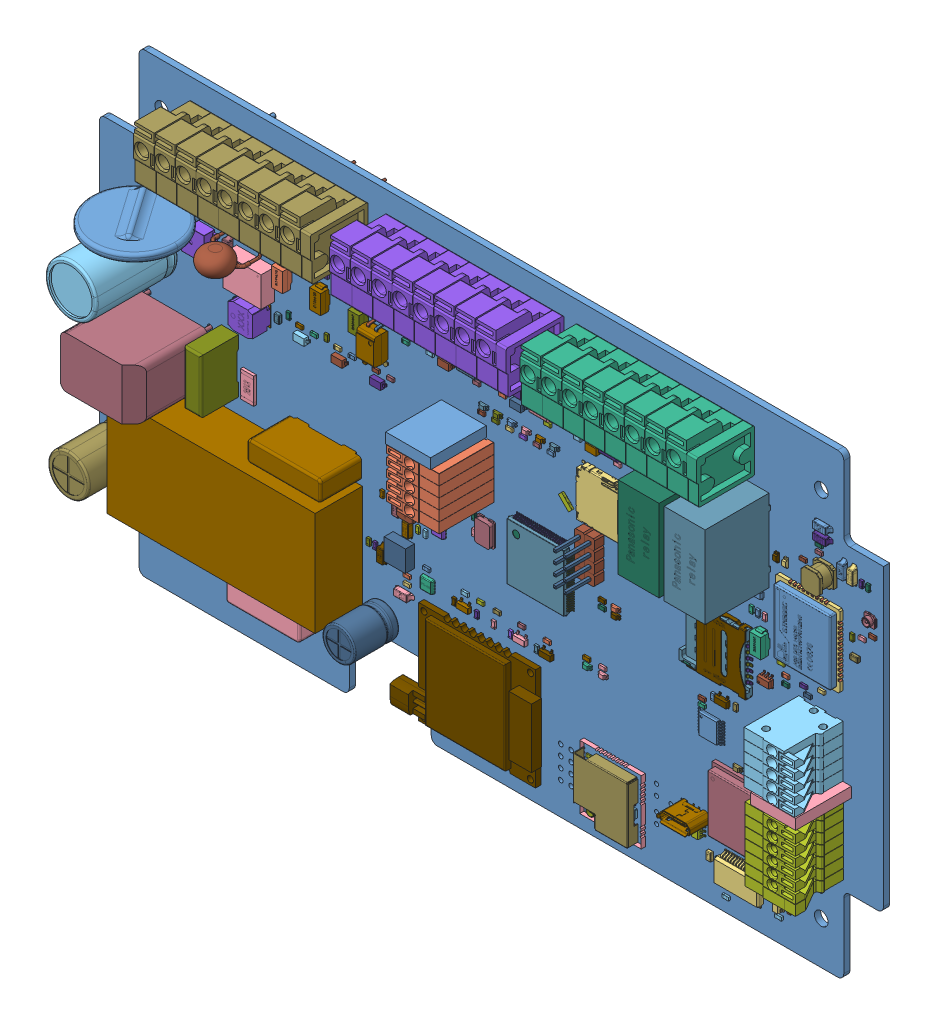
SolidWorks assembly Velvet_Controller_V1.2_2023, configuration Default. Lengths in mm. (continued)
Components (placement in the parent): (continued)
- Velvet_Controller_V1.2_2023(2)^Velvet_Controller_V1.2_2023-1: Velvet_Controller_V1.2_2023(2)^Velvet_Controller_V1.2_2023 [Default] at origin size (191.4 111.4 51.25) (virtual) (continued)
  - C4lr^Velvet_Controller_V1.2_2023(2)_Velvet_Controller_V1.2_2023-1: C4lr^Velvet_Controller_V1.2_2023(2)_Velvet_Controller_V1.2_2023 [Default] at origin size (1.6 0.8 0.5) (virtual)
    - CAP 0603 (1608)^C4lr_Velvet_Controller_V1.2_2023(2)_Velvet_Controller_V1.2_2023-1: CAP 0603 (1608)^C4lr_Velvet_Controller_V1.2_2023(2)_Velvet_Controller_V1.2_2023 [Default] at (130.48 19.301 -1.5) x (-1 0 0) z (0 -1 0) size (1.6 0.5 0.8) (virtual)
  - C4gs^Velvet_Controller_V1.2_2023(2)_Velvet_Controller_V1.2_2023-1: C4gs^Velvet_Controller_V1.2_2023(2)_Velvet_Controller_V1.2_2023 [Default] at origin size (0.8 1.6 0.5) (virtual)
    - CAP 0603 (1608)^C4gs_Velvet_Controller_V1.2_2023(2)_Velvet_Controller_V1.2_2023-1: CAP 0603 (1608)^C4gs_Velvet_Controller_V1.2_2023(2)_Velvet_Controller_V1.2_2023 [Default] at (176.025 78.275 -1.5) x (0 -1 0) z (1 0 0) size (1.6 0.5 0.8) (virtual)
  - C3wf^Velvet_Controller_V1.2_2023(2)_Velvet_Controller_V1.2_2023-1: C3wf^Velvet_Controller_V1.2_2023(2)_Velvet_Controller_V1.2_2023 [Default] at origin size (1.62 4.56 1.51) (virtual)
    - CAP 1206^C3wf_Velvet_Controller_V1.2_2023(2)_Velvet_Controller_V1.2_2023-1: CAP 1206^C3wf_Velvet_Controller_V1.2_2023(2)_Velvet_Controller_V1.2_2023 [Default] at (162.3 28.55 -1.5) x (0 1 0) z (0 0 -1) size (4.56 1.62 1.51) (virtual)
  - C3p^Velvet_Controller_V1.2_2023(2)_Velvet_Controller_V1.2_2023-1: C3p^Velvet_Controller_V1.2_2023(2)_Velvet_Controller_V1.2_2023 [Default] at origin size (8 8 28.5) (virtual)
    - ECA-1HM101B^C3p_Velvet_Controller_V1.2_2023(2)_Velvet_Controller_V1.2_2023-1: ECA-1HM101B^C3p_Velvet_Controller_V1.2_2023(2)_Velvet_Controller_V1.2_2023 [Default] at (69.9 20.9 0) x (0 -1 0) z (-1 0 0) size (8 28.5 8) (virtual)
  - C3mc^Velvet_Controller_V1.2_2023(2)_Velvet_Controller_V1.2_2023-1: C3mc^Velvet_Controller_V1.2_2023(2)_Velvet_Controller_V1.2_2023 [Default] at origin size (1.6 0.8 0.5) (virtual)
    - CAP 0603 (1608)^C3mc_Velvet_Controller_V1.2_2023(2)_Velvet_Controller_V1.2_2023-1: CAP 0603 (1608)^C3mc_Velvet_Controller_V1.2_2023(2)_Velvet_Controller_V1.2_2023 [Default] at (146.575 42.225 0) x (1 0 0) z (0 -1 0) size (1.6 0.5 0.8) (virtual)
  - C3lr^Velvet_Controller_V1.2_2023(2)_Velvet_Controller_V1.2_2023-1: C3lr^Velvet_Controller_V1.2_2023(2)_Velvet_Controller_V1.2_2023 [Default] at origin size (4.56 1.62 1.51) (virtual)
    - CAP 1206^C3lr_Velvet_Controller_V1.2_2023(2)_Velvet_Controller_V1.2_2023-1: CAP 1206^C3lr_Velvet_Controller_V1.2_2023(2)_Velvet_Controller_V1.2_2023 [Default] at (128.88 21.701 -1.5) x (1 0 0) z (0 0 -1) size (4.56 1.62 1.51) (virtual)
  - C3io^Velvet_Controller_V1.2_2023(2)_Velvet_Controller_V1.2_2023-1: C3io^Velvet_Controller_V1.2_2023(2)_Velvet_Controller_V1.2_2023 [Default] at origin size (1.6 0.8 0.5) (virtual)
    - CAP 0603 (1608)^C3io_Velvet_Controller_V1.2_2023(2)_Velvet_Controller_V1.2_2023-1: CAP 0603 (1608)^C3io_Velvet_Controller_V1.2_2023(2)_Velvet_Controller_V1.2_2023 [Default] at (70.58 71.8 0) x (1 0 0) z (0 -1 0) size (1.6 0.5 0.8) (virtual)
  - C3gs^Velvet_Controller_V1.2_2023(2)_Velvet_Controller_V1.2_2023-1: C3gs^Velvet_Controller_V1.2_2023(2)_Velvet_Controller_V1.2_2023 [Default] at origin size (0.8 1.6 0.5) (virtual)
    - CAP 0603 (1608)^C3gs_Velvet_Controller_V1.2_2023(2)_Velvet_Controller_V1.2_2023-1: CAP 0603 (1608)^C3gs_Velvet_Controller_V1.2_2023(2)_Velvet_Controller_V1.2_2023 [Default] at (174.425 78.275 -1.5) x (0 -1 0) z (1 0 0) size (1.6 0.5 0.8) (virtual)
  - C2wf^Velvet_Controller_V1.2_2023(2)_Velvet_Controller_V1.2_2023-1: C2wf^Velvet_Controller_V1.2_2023(2)_Velvet_Controller_V1.2_2023 [Default] at origin size (0.8 1.6 0.5) (virtual)
    - CAP 0603 (1608)^C2wf_Velvet_Controller_V1.2_2023(2)_Velvet_Controller_V1.2_2023-1: CAP 0603 (1608)^C2wf_Velvet_Controller_V1.2_2023(2)_Velvet_Controller_V1.2_2023 [Default] at (151.525 9.45 0) x (0 1 0) z (1 0 0) size (1.6 0.5 0.8) (virtual)
  - C2p^Velvet_Controller_V1.2_2023(2)_Velvet_Controller_V1.2_2023-1: C2p^Velvet_Controller_V1.2_2023(2)_Velvet_Controller_V1.2_2023 [Default] at origin size (4.21 13.2 36.1) (virtual)
    - CFR_RB2_13X9X4_L13.2H9.1T4.2S10LL27F0.65^C2p_Velvet_Controller_V1.2_2023(2)_Velvet_Controller_V1.2_2023-1: CFR_RB2_13X9X4_L13.2H9.1T4.2S10LL27F0.65^C2p_Velvet_Controller_V1.2_2023(2)_Velvet_Controller_V1.2_2023 [Default] at (33.9525 62.7 0) x (0 -1 0) z (-1 0 0) size (13.2 36.1 4.21) (virtual)
  - C2mc^Velvet_Controller_V1.2_2023(2)_Velvet_Controller_V1.2_2023-1: C2mc^Velvet_Controller_V1.2_2023(2)_Velvet_Controller_V1.2_2023 [Default] at origin size (0.8 1.6 0.5) (virtual)
    - CAP 0603 (1608)^C2mc_Velvet_Controller_V1.2_2023(2)_Velvet_Controller_V1.2_2023-1: CAP 0603 (1608)^C2mc_Velvet_Controller_V1.2_2023(2)_Velvet_Controller_V1.2_2023 [Default] at (97.35 50.05 -1.5) x (0 -1 0) z (1 0 0) size (1.6 0.5 0.8) (virtual)
  - C2lr^Velvet_Controller_V1.2_2023(2)_Velvet_Controller_V1.2_2023-1: C2lr^Velvet_Controller_V1.2_2023(2)_Velvet_Controller_V1.2_2023 [Default] at origin size (0.8 1.6 0.5) (virtual)
    - CAP 0603 (1608)^C2lr_Velvet_Controller_V1.2_2023(2)_Velvet_Controller_V1.2_2023-1: CAP 0603 (1608)^C2lr_Velvet_Controller_V1.2_2023(2)_Velvet_Controller_V1.2_2023 [Default] at (103.7 4.1 -1.5) x (0 1 0) z (-1 0 0) size (1.6 0.5 0.8) (virtual)
  - C2io^Velvet_Controller_V1.2_2023(2)_Velvet_Controller_V1.2_2023-1: C2io^Velvet_Controller_V1.2_2023(2)_Velvet_Controller_V1.2_2023 [Default] at origin size (1.6 0.8 0.5) (virtual)
    - CAP 0603 (1608)^C2io_Velvet_Controller_V1.2_2023(2)_Velvet_Controller_V1.2_2023-1: CAP 0603 (1608)^C2io_Velvet_Controller_V1.2_2023(2)_Velvet_Controller_V1.2_2023 [Default] at (61.21 71.8 0) x (1 0 0) z (0 -1 0) size (1.6 0.5 0.8) (virtual)
  - C2gs^Velvet_Controller_V1.2_2023(2)_Velvet_Controller_V1.2_2023-1: C2gs^Velvet_Controller_V1.2_2023(2)_Velvet_Controller_V1.2_2023 [Default] at origin size (1.25 2 0.78) (virtual)
    - CAP 0805^C2gs_Velvet_Controller_V1.2_2023(2)_Velvet_Controller_V1.2_2023-1: CAP 0805^C2gs_Velvet_Controller_V1.2_2023(2)_Velvet_Controller_V1.2_2023 [Default] at (172.225 77.275 -1.5) x (0 -1 0) z (1 0 0) size (2 0.78 1.25) (virtual)
  - C1wf^Velvet_Controller_V1.2_2023(2)_Velvet_Controller_V1.2_2023-1: C1wf^Velvet_Controller_V1.2_2023(2)_Velvet_Controller_V1.2_2023 [Default] at origin size (1.25 2 0.78) (virtual)
    - CAP 0805^C1wf_Velvet_Controller_V1.2_2023(2)_Velvet_Controller_V1.2_2023-1: CAP 0805^C1wf_Velvet_Controller_V1.2_2023(2)_Velvet_Controller_V1.2_2023 [Default] at (149.35 10.45 0) x (0 1 0) z (1 0 0) size (2 0.78 1.25) (virtual)
  - C1p^Velvet_Controller_V1.2_2023(2)_Velvet_Controller_V1.2_2023-1: C1p^Velvet_Controller_V1.2_2023(2)_Velvet_Controller_V1.2_2023 [Default] at origin size (18 5 16.5) (virtual)
    - B32^C1p_Velvet_Controller_V1.2_2023(2)_Velvet_Controller_V1.2_2023-1: B32^C1p_Velvet_Controller_V1.2_2023(2)_Velvet_Controller_V1.2_2023 [Default] at (50.3 17.6 5.5) x (1 0 0) z (0 -1 0) size (18 16.5 5) (virtual)
  - C1lr^Velvet_Controller_V1.2_2023(2)_Velvet_Controller_V1.2_2023-1: C1lr^Velvet_Controller_V1.2_2023(2)_Velvet_Controller_V1.2_2023 [Default] at origin size (1.62 4.56 1.51) (virtual)
    - CAP 1206^C1lr_Velvet_Controller_V1.2_2023(2)_Velvet_Controller_V1.2_2023-1: CAP 1206^C1lr_Velvet_Controller_V1.2_2023(2)_Velvet_Controller_V1.2_2023 [Default] at (107.6 6.1 -1.5) x (0 -1 0) z (0 0 -1) size (4.56 1.62 1.51) (virtual)
  - C1io^Velvet_Controller_V1.2_2023(2)_Velvet_Controller_V1.2_2023-1: C1io^Velvet_Controller_V1.2_2023(2)_Velvet_Controller_V1.2_2023 [Default] at origin size (1.6 0.8 0.5) (virtual)
    - CAP 0603 (1608)^C1io_Velvet_Controller_V1.2_2023(2)_Velvet_Controller_V1.2_2023-1: CAP 0603 (1608)^C1io_Velvet_Controller_V1.2_2023(2)_Velvet_Controller_V1.2_2023 [Default] at (51.91 71.8 0) x (1 0 0) z (0 -1 0) size (1.6 0.5 0.8) (virtual)
  - C1gs^Velvet_Controller_V1.2_2023(2)_Velvet_Controller_V1.2_2023-1: C1gs^Velvet_Controller_V1.2_2023(2)_Velvet_Controller_V1.2_2023 [Default] at origin size (4.45 7.41 3.01) (virtual)
    - 2917 TANTAL^C1gs_Velvet_Controller_V1.2_2023(2)_Velvet_Controller_V1.2_2023-1: 2917 TANTAL^C1gs_Velvet_Controller_V1.2_2023(2)_Velvet_Controller_V1.2_2023 [Default] at (179.05 75.55 -1.5) x (0 1 0) z (0 0 -1) size (7.41 4.45 3.01) (virtual)
